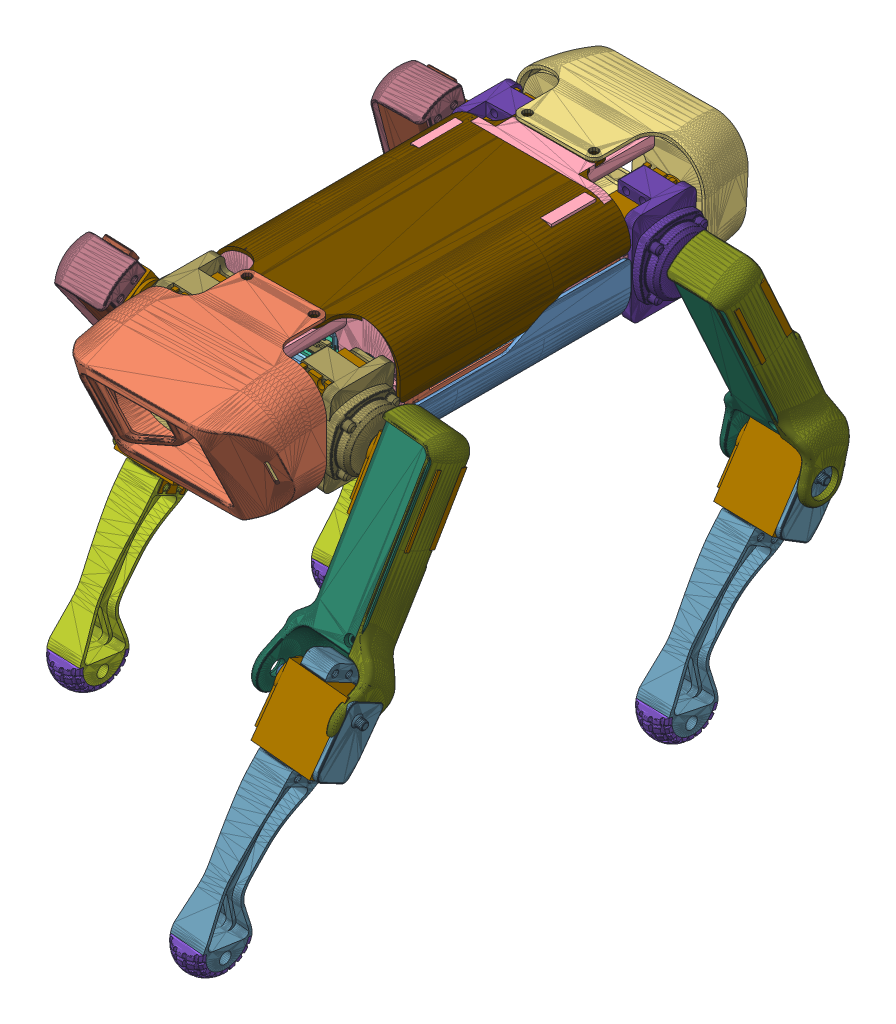
SolidWorks assembly robot_dog_jestson, configuration Default. Lengths in mm.
Overall size (261.86 298.31 449.5).
480 component instances, 93 part files, 20 mates.
Components (placement in the parent):
- torsol_with_jestson-1: torsol_with_jestson [Default] at (84.8958 -47.9637 220.9974) size (110.41 70.14 242.41)
  - R_side_plate-1: R_side_plate [Default] at (-145.3547 -0.5404 -42.0354) x (1 0 0) z (0 -1 0) size (6.5 130 29)
  - non-mega_L_side_plate_jetson-2: non-mega_L_side_plate_jetson [Default] at (-41.8547 39.5958 -42.0354) x (-1 0 0) z (0 1 0) size (6.5 130 29)
  - O_shoulder-1: O_shoulder [Default] at (-38.1905 81.6503 -93.0354) x (-1 0 0) z (0 -1 0) size (110 5.21 66)
  - I_shoulder_mg-1: I_shoulder_mg [Default] at (-38.6047 81.5958 -42.0354) x (-1 0 0) z (0 -1 0) size (110 51 70)
  - I_shoulder_mg-2: I_shoulder_mg [Default] at (-148.6047 81.4596 87.9646) x (1 0 0) z (0 -1 0) size (110 51 70)
  - O_shoulder-2: O_shoulder [Default] at (-148.6047 81.4596 138.9646) x (1 0 0) z (0 -1 0) size (110 5.21 66)
  - plate_with_jetson-1: plate_with_jetson [Default] at (-139.2728 38.0458 18.6623) x (-1 0 0) z (0 -1 0) size (107 130 44.9)
    - plate_jetson-1: plate_jetson [Default] at (-46.1681 -3.8023 -1.45) size (107 130 2.9)
    - Jetson nano_fixed.step-1: Jetson nano_fixed.step [Default] at (-69.1681 -65.6237 -1.45) x (0 1 0) z (0 0 -1) size (100 81.03 30.51)
      - 142-13449-1000-A02_ASM.step-1: 142-13449-1000-A02_ASM.step [Default] at origin size (100 81.03 23.19)
        - 142-13449-1000-A02.step-1: 142-13449-1000-A02.step [Default] at origin size (100 79 1.57)
        - 315-1109-000_1.step-1: 315-1109-000_1.step [Default] at (5.6 4.9 1.575) x (-1 0 0) z (0 0 1) size (4.5 3.5 0.8)
        - 0402_H040.step-1: 0402_H040.step [Default] at (8 -0.825 1.575) size (1 0.5 0.4)
        - 0402_H060.step-1: 0402_H060.step [Default] at (1 5 1.575) x (0 -1 0) z (0 0 1) size (1 0.5 0.6)
        - 0402_H040.step-2: 0402_H040.step [Default] at (9.9 -0.3 1.575) size (1 0.5 0.4)
        - 0402_H040.step-3: 0402_H040.step [Default] at (8.296 51.194 1.575) x (-1 0 0) z (0 0 1) size (1 0.5 0.4)
        - 0402_H040.step-4: 0402_H040.step [Default] at (76.2 36.9 1.575) x (-1 0 0) z (0 0 1) size (1 0.5 0.4)
        - 0402_H040.step-5: 0402_H040.step [Default] at (37.8 2.87 1.575) x (0 -1 0) z (0 0 1) size (1 0.5 0.4)
        - 0402_H040.step-6: 0402_H040.step [Default] at (38.6 2.87 1.575) x (0 -1 0) z (0 0 1) size (1 0.5 0.4)
        - 0402_H060.step-2: 0402_H060.step [Default] at (14.2 7.7 1.575) x (0 -1 0) z (0 0 1) size (1 0.5 0.6)
        - 0402_H040.step-7: 0402_H040.step [Default] at (64 27.5 1.575) x (-1 0 0) z (0 0 1) size (1 0.5 0.4)
        - 0402_H060.step-3: 0402_H060.step [Default] at (18.6 43.15 1.575) x (-1 0 0) z (0 0 1) size (1 0.5 0.6)
        - 0402_H060.step-4: 0402_H060.step [Default] at (65.5 52.8 1.575) x (0 1 0) z (0 0 1) size (1 0.5 0.6)
        - 0402_H060.step-5: 0402_H060.step [Default] at (64 28.4 1.575) x (-1 0 0) z (0 0 1) size (1 0.5 0.6)
        - 0402_H040.step-8: 0402_H040.step [Default] at (60.95 25.85 1.575) size (1 0.5 0.4)
        - 0402_H060.step-6: 0402_H060.step [Default] at (17.3 7.7 1.575) x (0 -1 0) z (0 0 1) size (1 0.5 0.6)
        - 0402_H060.step-7: 0402_H060.step [Default] at (18.6 7.7 1.575) x (0 -1 0) z (0 0 1) size (1 0.5 0.6)
        - 0402_H060.step-8: 0402_H060.step [Default] at (12.9 7.7 1.575) x (0 -1 0) z (0 0 1) size (1 0.5 0.6)
        - 0402_H060.step-9: 0402_H060.step [Default] at (80.9 37.7 1.575) x (-1 0 0) z (0 0 1) size (1 0.5 0.6)
        - 0402_H040.step-9: 0402_H040.step [Default] at (79.5 31.3 1.575) size (1 0.5 0.4)
        - 0402_H040.step-10: 0402_H040.step [Default] at (81 31.3 1.575) x (-1 0 0) z (0 0 1) size (1 0.5 0.4)
        - 0402_H060.step-10: 0402_H060.step [Default] at (79.3 37.7 1.575) size (1 0.5 0.6)
        - 0402_H060.step-11: 0402_H060.step [Default] at (74.8 4.05 1.575) x (-1 0 0) z (0 0 1) size (1 0.5 0.6)
        - 0402_H040.step-11: 0402_H040.step [Default] at (65.675 6.15 1.575) x (0 -1 0) z (0 0 1) size (1 0.5 0.4)
        - 0402_H060.step-12: 0402_H060.step [Default] at (67.7 6.85 1.575) x (0 1 0) z (0 0 1) size (1 0.5 0.6)
        - 0402_H040.step-12: 0402_H040.step [Default] at (64.475 5.8 1.575) x (-1 0 0) z (0 0 1) size (1 0.5 0.4)
        - 0402_H040.step-13: 0402_H040.step [Default] at (67.725 5.325 1.575) x (0 1 0) z (0 0 1) size (1 0.5 0.4)
        - 0402_H060.step-13: 0402_H060.step [Default] at (46.1 59.45 1.575) size (1 0.5 0.6)
        - 0402_H040.step-14: 0402_H040.step [Default] at (44.65 59.45 1.575) size (1 0.5 0.4)
        - 0402_H040.step-15: 0402_H040.step [Default] at (46.1 60.25 1.575) size (1 0.5 0.4)
        - 0402_H060.step-14: 0402_H060.step [Default] at (53.35 57.7 1.575) x (0 -1 0) z (0 0 1) size (1 0.5 0.6)
        - 0402_H040.step-16: 0402_H040.step [Default] at (47.6 59.45 1.575) size (1 0.5 0.4)
        - 0402_H040.step-17: 0402_H040.step [Default] at (48.4 60.25 1.575) size (1 0.5 0.4)
        - 0402_H040.step-18: 0402_H040.step [Default] at (47.7 58.325 1.575) x (0 1 0) z (0 0 1) size (1 0.5 0.4)
        - 0402_H060.step-15: 0402_H060.step [Default] at (46.5 58.65 1.575) x (-1 0 0) z (0 0 1) size (1 0.5 0.6)
        - 0402_H060.step-16: 0402_H060.step [Default] at (51.8 60.25 1.575) size (1 0.5 0.6)
        - 0402_H040.step-19: 0402_H040.step [Default] at (53.35 59.4 1.575) x (0 -1 0) z (0 0 1) size (1 0.5 0.4)
        - 0402_H040.step-20: 0402_H040.step [Default] at (50.2 60.25 1.575) x (-1 0 0) z (0 0 1) size (1 0.5 0.4)
        - 0402_H060.step-17: 0402_H060.step [Default] at (18.6 43.95 1.575) x (-1 0 0) z (0 0 1) size (1 0.5 0.6)
        - 0402_H060.step-18: 0402_H060.step [Default] at (52.75 2.9 1.575) x (0 -1 0) z (0 0 1) size (1 0.5 0.6)
        - 0402_H060.step-19: 0402_H060.step [Default] at (22.35 47.4 1.575) x (-1 0 0) z (0 0 1) size (1 0.5 0.6)
        - 0402_H060.step-20: 0402_H060.step [Default] at (20.55 47.4 1.575) x (-1 0 0) z (0 0 1) size (1 0.5 0.6)
        - 0402_H060.step-21: 0402_H060.step [Default] at (21.95 34.55 1.575) x (0 -1 0) z (0 0 1) size (1 0.5 0.6)
        - 0402_H060.step-22: 0402_H060.step [Default] at (21.05 34.55 1.575) x (0 -1 0) z (0 0 1) size (1 0.5 0.6)
        - 0402_H060.step-23: 0402_H060.step [Default] at (53.55 2.9 1.575) x (0 -1 0) z (0 0 1) size (1 0.5 0.6)
        - 0402_H060.step-24: 0402_H060.step [Default] at (25.4 54 1.575) x (-1 0 0) z (0 0 1) size (1 0.5 0.6)
        - 0402_H060.step-25: 0402_H060.step [Default] at (24 34.58 1.575) x (0 -1 0) z (0 0 1) size (1 0.5 0.6)
        - 0402_H040.step-21: 0402_H040.step [Default] at (55.6 2.95 1.575) x (0 -1 0) z (0 0 1) size (1 0.5 0.4)
        - 0402_H040.step-22: 0402_H040.step [Default] at (20.13 34.53 1.575) x (0 1 0) z (0 0 1) size (1 0.5 0.4)
        - 0402_H060.step-26: 0402_H060.step [Default] at (18.4 35.15 1.575) x (0 1 0) z (0 0 1) size (1 0.5 0.6)
        - 0402_H060.step-27: 0402_H060.step [Default] at (18.4 36.75 1.575) x (0 1 0) z (0 0 1) size (1 0.5 0.6)
        - 0402_H040.step-23: 0402_H040.step [Default] at (39.6 2.87 1.575) x (0 -1 0) z (0 0 1) size (1 0.5 0.4)
        - 0402_H040.step-24: 0402_H040.step [Default] at (40.4 2.87 1.575) x (0 -1 0) z (0 0 1) size (1 0.5 0.4)
        - 0402_H040.step-25: 0402_H040.step [Default] at (60.95 2.95 1.575) x (0 -1 0) z (0 0 1) size (1 0.5 0.4)
        - 0402_H040.step-26: 0402_H040.step [Default] at (60.15 2.95 1.575) x (0 -1 0) z (0 0 1) size (1 0.5 0.4)
        - 0402_H040.step-27: 0402_H040.step [Default] at (54.8 2.95 1.575) x (0 -1 0) z (0 0 1) size (1 0.5 0.4)
        - 0402_H040.step-28: 0402_H040.step [Default] at (31.6 54 1.575) size (1 0.5 0.4)
        - 0402_H040.step-29: 0402_H040.step [Default] at (27.4 54 1.575) size (1 0.5 0.4)
        - 0402_H040.step-30: 0402_H040.step [Default] at (29.6 54 1.575) x (-1 0 0) z (0 0 1) size (1 0.5 0.4)
        - 0402_H040.step-31: 0402_H040.step [Default] at (63.775 -14.475 1.575) size (1 0.5 0.4)
        - 0402_H040.step-32: 0402_H040.step [Default] at (63.775 -15.275 1.575) size (1 0.5 0.4)
        - 0402_H040.step-33: 0402_H040.step [Default] at (8.025 41.475 1.575) x (-1 0 0) z (0 0 1) size (1 0.5 0.4)
        - 0402_H060.step-28: 0402_H060.step [Default] at (63.95 1.25 1.575) x (0 1 0) z (0 0 1) size (1 0.5 0.6)
        - 0402_H060.step-29: 0402_H060.step [Default] at (2.95 54.05 1.575) x (0 1 0) z (0 0 1) size (1 0.5 0.6)
        - 0402_H040.step-34: 0402_H040.step [Default] at (92.2 -3.45 1.575) x (-1 0 0) z (0 0 1) size (1 0.5 0.4)
        - 0402_H060.step-30: 0402_H060.step [Default] at (32.85 7.7 1.575) x (0 -1 0) z (0 0 1) size (1 0.5 0.6)
        - 0402_H060.step-31: 0402_H060.step [Default] at (27.25 7.7 1.575) x (0 -1 0) z (0 0 1) size (1 0.5 0.6)
        - 0402_H060.step-32: 0402_H060.step [Default] at (31.25 7.7 1.575) x (0 -1 0) z (0 0 1) size (1 0.5 0.6)
        - 0402_H060.step-33: 0402_H060.step [Default] at (28.85 7.7 1.575) x (0 -1 0) z (0 0 1) size (1 0.5 0.6)
        - 0402_H060.step-34: 0402_H060.step [Default] at (32.05 7.7 1.575) x (0 -1 0) z (0 0 1) size (1 0.5 0.6)
        - 0402_H060.step-35: 0402_H060.step [Default] at (28.05 7.7 1.575) x (0 -1 0) z (0 0 1) size (1 0.5 0.6)
        - 0402_H060.step-36: 0402_H060.step [Default] at (30.45 7.7 1.575) x (0 -1 0) z (0 0 1) size (1 0.5 0.6)
        - 0402_H060.step-37: 0402_H060.step [Default] at (29.65 7.7 1.575) x (0 -1 0) z (0 0 1) size (1 0.5 0.6)
        - 0402_H060.step-38: 0402_H060.step [Default] at (24.65 6.41 1.575) x (0 -1 0) z (0 0 1) size (1 0.5 0.6)
        - 0402_H060.step-39: 0402_H060.step [Default] at (25.85 6.41 1.575) x (0 -1 0) z (0 0 1) size (1 0.5 0.6)
        - 0402_H060.step-40: 0402_H060.step [Default] at (4.2 36.5 1.575) x (0 1 0) z (0 0 1) size (1 0.5 0.6)
        - 0402_H060.step-41: 0402_H060.step [Default] at (89.7 4.7 1.575) x (0 -1 0) z (0 0 1) size (1 0.5 0.6)
        - 0402_H060.step-42: 0402_H060.step [Default] at (82.5 3.8 1.575) x (0 -1 0) z (0 0 1) size (1 0.5 0.6)
        - 0402_H060.step-43: 0402_H060.step [Default] at (12.65 49.7 1.575) size (1 0.5 0.6)
        - 0402_H060.step-44: 0402_H060.step [Default] at (11.2 50.15 1.575) x (0 -1 0) z (0 0 1) size (1 0.5 0.6)
        - 0402_H060.step-45: 0402_H060.step [Default] at (26.5 34.55 1.575) x (0 -1 0) z (0 0 1) size (1 0.5 0.6)
        - 0402_H060.step-46: 0402_H060.step [Default] at (29.9 34.5 1.575) x (0 -1 0) z (0 0 1) size (1 0.5 0.6)
        - 0402_H060.step-47: 0402_H060.step [Default] at (31.7 40.15 1.575) x (0 1 0) z (0 0 1) size (1 0.5 0.6)
        - 0402_H060.step-48: 0402_H060.step [Default] at (31.15 42.5 1.575) x (0 1 0) z (0 0 1) size (1 0.5 0.6)
        - 0402_H060.step-49: 0402_H060.step [Default] at (19.2 47.05 1.575) x (0 1 0) z (0 0 1) size (1 0.5 0.6)
        - 0402_H060.step-50: 0402_H060.step [Default] at (17.95 42 1.575) x (0 -1 0) z (0 0 1) size (1 0.5 0.6)
        - 0402_H060.step-51: 0402_H060.step [Default] at (27.3 48.25 1.575) x (0 1 0) z (0 0 1) size (1 0.5 0.6)
        - 0402_H060.step-52: 0402_H060.step [Default] at (31.7 37.85 1.575) x (0 -1 0) z (0 0 1) size (1 0.5 0.6)
        - 0402_H060.step-53: 0402_H060.step [Default] at (29.6 48.35 1.575) x (0 1 0) z (0 0 1) size (1 0.5 0.6)
        - 0402_H060.step-54: 0402_H060.step [Default] at (18.8 38.75 1.575) x (-1 0 0) z (0 0 1) size (1 0.5 0.6)
        - 0402_H060.step-55: 0402_H060.step [Default] at (18.7 57.2 1.575) x (0 -1 0) z (0 0 1) size (1 0.5 0.6)
        - 0402_H060.step-56: 0402_H060.step [Default] at (34.1 2.9 1.575) x (0 -1 0) z (0 0 1) size (1 0.5 0.6)
        - 0402_H060.step-57: 0402_H060.step [Default] at (35.8 2.9 1.575) x (0 -1 0) z (0 0 1) size (1 0.5 0.6)
        - 0402_H060.step-58: 0402_H060.step [Default] at (34.9 2.9 1.575) x (0 -1 0) z (0 0 1) size (1 0.5 0.6)
        - 0402_H060.step-59: 0402_H060.step [Default] at (36.6 2.9 1.575) x (0 -1 0) z (0 0 1) size (1 0.5 0.6)
        - 0402_H060.step-60: 0402_H060.step [Default] at (11.325 44.725 1.575) size (1 0.5 0.6)
        - 0402_H060.step-61: 0402_H060.step [Default] at (50.95 2.9 1.575) x (0 -1 0) z (0 0 1) size (1 0.5 0.6)
        - 0402_H060.step-62: 0402_H060.step [Default] at (51.75 2.9 1.575) x (0 -1 0) z (0 0 1) size (1 0.5 0.6)
        - 0402_H060.step-63: 0402_H060.step [Default] at (11.55 39.7 1.575) size (1 0.5 0.6)
        - 0402_H060.step-64: 0402_H060.step [Default] at (9.5 -8.5 1.575) x (-1 0 0) z (0 0 1) size (1 0.5 0.6)
        - 0402_H060.step-65: 0402_H060.step [Default] at (61.35 38.05 1.575) x (0 -1 0) z (0 0 1) size (1 0.5 0.6)
        - 0402_H060.step-66: 0402_H060.step [Default] at (60.55 38.05 1.575) x (0 -1 0) z (0 0 1) size (1 0.5 0.6)
        - 0402_H060.step-67: 0402_H060.step [Default] at (29.3 25.65 1.575) x (0 -1 0) z (0 0 1) size (1 0.5 0.6)
        - 0402_H060.step-68: 0402_H060.step [Default] at (63.3 56.2 1.575) x (0 1 0) z (0 0 1) size (1 0.5 0.6)
        - 0402_H060.step-69: 0402_H060.step [Default] at (20.5 54.2 1.575) size (1 0.5 0.6)
        - 0402_H060.step-70: 0402_H060.step [Default] at (60.1 32.15 1.575) x (0 1 0) z (0 0 1) size (1 0.5 0.6)
        - 0402_H060.step-71: 0402_H060.step [Default] at (60.9 32.15 1.575) x (0 1 0) z (0 0 1) size (1 0.5 0.6)
        - 0402_H060.step-72: 0402_H060.step [Default] at (18.6 44.85 1.575) size (1 0.5 0.6)
        - 0402_H060.step-73: 0402_H060.step [Default] at (18.6 45.65 1.575) size (1 0.5 0.6)
        - 0402_H060.step-74: 0402_H060.step [Default] at (18.1 27.25 1.575) size (1 0.5 0.6)
        - 0402_H060.step-75: 0402_H060.step [Default] at (15.1 7.7 1.575) x (0 -1 0) z (0 0 1) size (1 0.5 0.6)
        - 0402_H060.step-76: 0402_H060.step [Default] at (16.4 7.7 1.575) x (0 -1 0) z (0 0 1) size (1 0.5 0.6)
        - 0402_H060.step-77: 0402_H060.step [Default] at (20.8 7.7 1.575) x (0 -1 0) z (0 0 1) size (1 0.5 0.6)
        - 0402_H060.step-78: 0402_H060.step [Default] at (19.5 7.7 1.575) x (0 -1 0) z (0 0 1) size (1 0.5 0.6)
        - 0402_H060.step-79: 0402_H060.step [Default] at (21.9 2.8 1.575) size (1 0.5 0.6)
        - 0402_H060.step-80: 0402_H060.step [Default] at (12.75 29 1.575) size (1 0.5 0.6)
        - 0402_H060.step-81: 0402_H060.step [Default] at (10.225 5.1 1.575) size (1 0.5 0.6)
        - 0402_H060.step-82: 0402_H060.step [Default] at (22.8 27.65 1.575) x (0 1 0) z (0 0 1) size (1 0.5 0.6)
        - 0402_H060.step-83: 0402_H060.step [Default] at (18.85 25.15 1.575) x (0 -1 0) z (0 0 1) size (1 0.5 0.6)
        - 0402_H060.step-84: 0402_H060.step [Default] at (17.95 40.1 1.575) x (0 1 0) z (0 0 1) size (1 0.5 0.6)
        - 0402_H040.step-35: 0402_H040.step [Default] at (20.8 6.2 1.575) x (0 1 0) z (0 0 1) size (1 0.5 0.4)
        - 0402_H040.step-36: 0402_H040.step [Default] at (76 22.7 1.575) size (1 0.5 0.4)
        - 0402_H040.step-37: 0402_H040.step [Default] at (23.7 26.85 1.575) x (0 1 0) z (0 0 1) size (1 0.5 0.4)
        - 0402_H040.step-38: 0402_H040.step [Default] at (18 25.15 1.575) x (0 1 0) z (0 0 1) size (1 0.5 0.4)
        - 0402_H040.step-39: 0402_H040.step [Default] at (17.3 28.25 1.575) x (-1 0 0) z (0 0 1) size (1 0.5 0.4)
        - 0402_H040.step-40: 0402_H040.step [Default] at (13.15 4.2 1.575) x (0 -1 0) z (0 0 1) size (1 0.5 0.4)
        - 0402_H040.step-41: 0402_H040.step [Default] at (17.2 30.15 1.575) x (0 -1 0) z (0 0 1) size (1 0.5 0.4)
        - 0402_H040.step-42: 0402_H040.step [Default] at (14.2 6.2 1.575) x (0 1 0) z (0 0 1) size (1 0.5 0.4)
        - 0402_H040.step-43: 0402_H040.step [Default] at (12.9 6.2 1.575) x (0 1 0) z (0 0 1) size (1 0.5 0.4)
        - 0402_H040.step-44: 0402_H040.step [Default] at (15.1 6.2 1.575) x (0 1 0) z (0 0 1) size (1 0.5 0.4)
        - 0402_H040.step-45: 0402_H040.step [Default] at (16.4 6.2 1.575) x (0 1 0) z (0 0 1) size (1 0.5 0.4)
        - 0402_H040.step-46: 0402_H040.step [Default] at (19.5 6.2 1.575) x (0 1 0) z (0 0 1) size (1 0.5 0.4)
        - 0402_H040.step-47: 0402_H040.step [Default] at (17.3 6.2 1.575) x (0 1 0) z (0 0 1) size (1 0.5 0.4)
        - 0402_H040.step-48: 0402_H040.step [Default] at (18.6 6.2 1.575) x (0 1 0) z (0 0 1) size (1 0.5 0.4)
        - 0402_H040.step-49: 0402_H040.step [Default] at (24.2 24.55 1.575) x (0 1 0) z (0 0 1) size (1 0.5 0.4)
        - 0402_H040.step-50: 0402_H040.step [Default] at (23.5 54.9 1.575) x (0 1 0) z (0 0 1) size (1 0.5 0.4)
        - 0402_H040.step-51: 0402_H040.step [Default] at (13.2 39.75 1.575) x (-1 0 0) z (0 0 1) size (1 0.5 0.4)
        - 0402_H040.step-52: 0402_H040.step [Default] at (80.7 47.4 1.575) x (-1 0 0) z (0 0 1) size (1 0.5 0.4)
        - 0402_H040.step-53: 0402_H040.step [Default] at (77.5 22.7 1.575) x (-1 0 0) z (0 0 1) size (1 0.5 0.4)
        - 0402_H040.step-54: 0402_H040.step [Default] at (9.25 -12.75 1.575) x (-1 0 0) z (0 0 1) size (1 0.5 0.4)
        - 0402_H040.step-55: 0402_H040.step [Default] at (9.25 -11.95 1.575) x (-1 0 0) z (0 0 1) size (1 0.5 0.4)
        - 0402_H040.step-56: 0402_H040.step [Default] at (64.475 6.7 1.575) size (1 0.5 0.4)
        - 0402_H040.step-57: 0402_H040.step [Default] at (29.3 24 1.575) x (0 1 0) z (0 0 1) size (1 0.5 0.4)
        - 0402_H040.step-58: 0402_H040.step [Default] at (64.2 32.5 1.575) x (0 1 0) z (0 0 1) size (1 0.5 0.4)
        - 0402_H040.step-59: 0402_H040.step [Default] at (64.15 47.45 1.575) x (0 -1 0) z (0 0 1) size (1 0.5 0.4)
        - 0402_H040.step-60: 0402_H040.step [Default] at (64.2 31 1.575) x (0 -1 0) z (0 0 1) size (1 0.5 0.4)
        - 0402_H040.step-61: 0402_H040.step [Default] at (76.2 36.1 1.575) x (-1 0 0) z (0 0 1) size (1 0.5 0.4)
        - 0402_H040.step-62: 0402_H040.step [Default] at (78.4 45.15 1.575) size (1 0.5 0.4)
        - 0402_H040.step-63: 0402_H040.step [Default] at (81.7 38.6 1.575) size (1 0.5 0.4)
        - 0402_H040.step-64: 0402_H040.step [Default] at (81.7 39.4 1.575) size (1 0.5 0.4)
        - 0402_H040.step-65: 0402_H040.step [Default] at (59.35 51.825 1.575) size (1 0.5 0.4)
        - 0402_H040.step-66: 0402_H040.step [Default] at (60.825 51.825 1.575) x (-1 0 0) z (0 0 1) size (1 0.5 0.4)
        - 0402_H040.step-67: 0402_H040.step [Default] at (89.7 9.5 1.575) x (0 1 0) z (0 0 1) size (1 0.5 0.4)
        - 0402_H040.step-68: 0402_H040.step [Default] at (89.7 6.7 1.575) x (0 1 0) z (0 0 1) size (1 0.5 0.4)
        - 0402_H040.step-69: 0402_H040.step [Default] at (3.9 34.2 1.575) x (0 -1 0) z (0 0 1) size (1 0.5 0.4)
        - 0402_H040.step-70: 0402_H040.step [Default] at (5.1 35 1.575) x (0 1 0) z (0 0 1) size (1 0.5 0.4)
        - 0402_H040.step-71: 0402_H040.step [Default] at (32.85 5.81 1.575) x (0 -1 0) z (0 0 1) size (1 0.5 0.4)
        - 0402_H040.step-72: 0402_H040.step [Default] at (32.05 5.81 1.575) x (0 -1 0) z (0 0 1) size (1 0.5 0.4)
        - 0402_H040.step-73: 0402_H040.step [Default] at (27.25 5.81 1.575) x (0 -1 0) z (0 0 1) size (1 0.5 0.4)
        - 0402_H040.step-74: 0402_H040.step [Default] at (28.05 5.81 1.575) x (0 -1 0) z (0 0 1) size (1 0.5 0.4)
        - 0402_H040.step-75: 0402_H040.step [Default] at (31.25 5.81 1.575) x (0 -1 0) z (0 0 1) size (1 0.5 0.4)
        - 0402_H040.step-76: 0402_H040.step [Default] at (30.45 5.81 1.575) x (0 -1 0) z (0 0 1) size (1 0.5 0.4)
        - 0402_H040.step-77: 0402_H040.step [Default] at (28.85 5.81 1.575) x (0 -1 0) z (0 0 1) size (1 0.5 0.4)
        - 0402_H040.step-78: 0402_H040.step [Default] at (29.65 5.81 1.575) x (0 -1 0) z (0 0 1) size (1 0.5 0.4)
        - 0402_H040.step-79: 0402_H040.step [Default] at (13.5 52.9 1.575) x (-1 0 0) z (0 0 1) size (1 0.5 0.4)
        - 0402_H040.step-80: 0402_H040.step [Default] at (22.35 4 1.575) x (0 -1 0) z (0 0 1) size (1 0.5 0.4)
        - 0402_H040.step-81: 0402_H040.step [Default] at (21.55 4 1.575) x (0 1 0) z (0 0 1) size (1 0.5 0.4)
        - 0402_H040.step-82: 0402_H040.step [Default] at (25.85 4.9 1.575) x (0 -1 0) z (0 0 1) size (1 0.5 0.4)
        - 0402_H040.step-83: 0402_H040.step [Default] at (11.8 52.9 1.575) size (1 0.5 0.4)
        - 0402_H040.step-84: 0402_H040.step [Default] at (9.432 51.594 1.575) x (0 -1 0) z (0 0 1) size (1 0.5 0.4)
        - 0402_H040.step-85: 0402_H040.step [Default] at (8.975 50.3 1.575) size (1 0.5 0.4)
        - 0402_H040.step-86: 0402_H040.step [Default] at (82.8 -5.3 1.575) x (-1 0 0) z (0 0 1) size (1 0.5 0.4)
        - 0402_H040.step-87: 0402_H040.step [Default] at (82.4 -11.6 1.575) x (-1 0 0) z (0 0 1) size (1 0.5 0.4)
        - 0402_H040.step-88: 0402_H040.step [Default] at (22.8 26.05 1.575) x (0 1 0) z (0 0 1) size (1 0.5 0.4)
        - 0402_H040.step-89: 0402_H040.step [Default] at (20.8 28.25 1.575) size (1 0.5 0.4)
        - 0402_H040.step-90: 0402_H040.step [Default] at (20.8 24.65 1.575) x (-1 0 0) z (0 0 1) size (1 0.5 0.4)
        - 0402_H040.step-91: 0402_H040.step [Default] at (18.1 26.45 1.575) size (1 0.5 0.4)
        - 0402_H040.step-92: 0402_H040.step [Default] at (24.65 8.41 1.575) x (0 1 0) z (0 0 1) size (1 0.5 0.4)
        - 0402_H040.step-93: 0402_H040.step [Default] at (25.85 8.41 1.575) x (0 1 0) z (0 0 1) size (1 0.5 0.4)
        - 0402_H040.step-94: 0402_H040.step [Default] at (3.8 54.4 1.575) x (0 -1 0) z (0 0 1) size (1 0.5 0.4)
        - 0402_H040.step-95: 0402_H040.step [Default] at (2.45 44.45 1.575) x (0 -1 0) z (0 0 1) size (1 0.5 0.4)
        - 0402_H040.step-96: 0402_H040.step [Default] at (24.65 4.9 1.575) x (0 1 0) z (0 0 1) size (1 0.5 0.4)
        - 0402_H040.step-97: 0402_H040.step [Default] at (22.15 7.6 1.575) x (-1 0 0) z (0 0 1) size (1 0.5 0.4)
        - 0402_H040.step-98: 0402_H040.step [Default] at (79.2 47.4 1.575) size (1 0.5 0.4)
        - 0402_H040.step-99: 0402_H040.step [Default] at (19 28.25 1.575) size (1 0.5 0.4)
        - 0402_H040.step-100: 0402_H040.step [Default] at (9.65 9.7 1.575) x (0 -1 0) z (0 0 1) size (1 0.5 0.4)
        - 0402_H040.step-101: 0402_H040.step [Default] at (28.35 34.45 1.575) x (0 1 0) z (0 0 1) size (1 0.5 0.4)
        - 0402_H040.step-102: 0402_H040.step [Default] at (25.2 34.55 1.575) x (0 1 0) z (0 0 1) size (1 0.5 0.4)
        - 0402_H040.step-103: 0402_H040.step [Default] at (10.625 6.35 1.575) x (0 -1 0) z (0 0 1) size (1 0.5 0.4)
        - 0402_H040.step-104: 0402_H040.step [Default] at (9.825 6.35 1.575) x (0 1 0) z (0 0 1) size (1 0.5 0.4)
        - 0402_H040.step-105: 0402_H040.step [Default] at (4.775 42.975 1.575) x (0 1 0) z (0 0 1) size (1 0.5 0.4)
        - 0402_H040.step-106: 0402_H040.step [Default] at (19.8 32.9 1.575) x (-1 0 0) z (0 0 1) size (1 0.5 0.4)
        - 0402_H040.step-107: 0402_H040.step [Default] at (22.35 24.65 1.575) x (-1 0 0) z (0 0 1) size (1 0.5 0.4)
        - 0402_H040.step-108: 0402_H040.step [Default] at (62.4 54.7 1.575) size (1 0.5 0.4)
        - 0402_H040.step-109: 0402_H040.step [Default] at (62.2 60.05 1.575) x (-1 0 0) z (0 0 1) size (1 0.5 0.4)
        - 0402_H040.step-110: 0402_H040.step [Default] at (23.5 57.5 1.575) x (0 1 0) z (0 0 1) size (1 0.5 0.4)
        - 0402_H040.step-111: 0402_H040.step [Default] at (12.8 44.725 1.575) size (1 0.5 0.4)
        - 0402_H040.step-112: 0402_H040.step [Default] at (21.8 31.45 1.575) x (0 1 0) z (0 0 1) size (1 0.5 0.4)
        - 0402_H040.step-113: 0402_H040.step [Default] at (19.25 34.55 1.575) x (0 1 0) z (0 0 1) size (1 0.5 0.4)
        - 0402_H040.step-114: 0402_H040.step [Default] at (0.95 41.55 1.575) size (1 0.5 0.4)
        - 0402_H040.step-115: 0402_H040.step [Default] at (64.1 58 1.575) x (0 1 0) z (0 0 1) size (1 0.5 0.4)
        - 0402_H040.step-116: 0402_H040.step [Default] at (63.3 58 1.575) x (0 -1 0) z (0 0 1) size (1 0.5 0.4)
        - 0402_H040.step-117: 0402_H040.step [Default] at (63.55 59.7 1.575) x (0 -1 0) z (0 0 1) size (1 0.5 0.4)
        - 0402_H060.step-85: 0402_H060.step [Default] at (71.175 4 1.575) x (-1 0 0) z (0 0 1) size (1 0.5 0.6)
        - 0402_H040.step-118: 0402_H040.step [Default] at (86.6 -5.6 1.575) x (0 1 0) z (0 0 1) size (1 0.5 0.4)
        - 0402_H040.step-119: 0402_H040.step [Default] at (85.8 -5.3 1.575) x (0 1 0) z (0 0 1) size (1 0.5 0.4)
        - 0402_H040.step-120: 0402_H040.step [Default] at (10.25 51.6 1.575) x (0 1 0) z (0 0 1) size (1 0.5 0.4)
        - 0402_H040.step-121: 0402_H040.step [Default] at (80.5 28.55 1.575) size (1 0.5 0.4)
        - 0402_H040.step-122: 0402_H040.step [Default] at (13.95 4.2 1.575) x (0 -1 0) z (0 0 1) size (1 0.5 0.4)
        - 0402_H040.step-123: 0402_H040.step [Default] at (15.35 4.2 1.575) x (0 -1 0) z (0 0 1) size (1 0.5 0.4)
        - 0402_H040.step-124: 0402_H040.step [Default] at (16.15 4.2 1.575) x (0 -1 0) z (0 0 1) size (1 0.5 0.4)
        - 0402_H040.step-125: 0402_H040.step [Default] at (20.55 4.2 1.575) x (0 -1 0) z (0 0 1) size (1 0.5 0.4)
        - 0402_H040.step-126: 0402_H040.step [Default] at (19.75 4.2 1.575) x (0 -1 0) z (0 0 1) size (1 0.5 0.4)
        - 0402_H040.step-127: 0402_H040.step [Default] at (17.6 4.2 1.575) x (0 -1 0) z (0 0 1) size (1 0.5 0.4)
        - 0402_H040.step-128: 0402_H040.step [Default] at (18.4 4.2 1.575) x (0 -1 0) z (0 0 1) size (1 0.5 0.4)
        - 0402_H060.step-86: 0402_H060.step [Default] at (64.25 -13.325 1.575) x (0 -1 0) z (0 0 1) size (1 0.5 0.6)
        - 0402_H060.step-87: 0402_H060.step [Default] at (64.225 -11.825 1.575) x (0 1 0) z (0 0 1) size (1 0.5 0.6)
        - 0402_H040.step-129: 0402_H040.step [Default] at (63.8 -6.85 1.575) x (0 1 0) z (0 0 1) size (1 0.5 0.4)
        - 0402_H040.step-130: 0402_H040.step [Default] at (81.7 41.95 1.575) size (1 0.5 0.4)
        - 0402_H040.step-131: 0402_H040.step [Default] at (87.75 -6 1.575) x (-1 0 0) z (0 0 1) size (1 0.5 0.4)
        - 0402_H040.step-132: 0402_H040.step [Default] at (82.4 -13.6 1.575) x (-1 0 0) z (0 0 1) size (1 0.5 0.4)
        - 0402_H060.step-88: 0402_H060.step [Default] at (91.75 -5.95 1.575) size (1 0.5 0.6)
        - 0402_H040.step-133: 0402_H040.step [Default] at (3.65 49.25 1.575) x (0 -1 0) z (0 0 1) size (1 0.5 0.4)
        - 0402_H040.step-134: 0402_H040.step [Default] at (2.45 49.25 1.575) x (0 1 0) z (0 0 1) size (1 0.5 0.4)
        - 0402_H040.step-135: 0402_H040.step [Default] at (90.75 -1.45 1.575) x (-1 0 0) z (0 0 1) size (1 0.5 0.4)
        - 0402_H040.step-136: 0402_H040.step [Default] at (8.45 39.55 1.575) x (0 -1 0) z (0 0 1) size (1 0.5 0.4)
        - 0402_H060.step-89: 0402_H060.step [Default] at (8.85 -5.25 1.575) x (-1 0 0) z (0 0 1) size (1 0.5 0.6)
        - 0402_H040.step-137: 0402_H040.step [Default] at (18.6 32.55 1.575) x (0 1 0) z (0 0 1) size (1 0.5 0.4)
        - 0402_H060.step-90: 0402_H060.step [Default] at (4.5 44.45 1.575) x (0 1 0) z (0 0 1) size (1 0.5 0.6)
        - 0402_H040.step-138: 0402_H040.step [Default] at (8.35 2.75 1.575) size (1 0.5 0.4)
        - 0402_H040.step-139: 0402_H040.step [Default] at (9.4 1.95 1.575) size (1 0.5 0.4)
        - 0402_H040.step-140: 0402_H040.step [Default] at (8.2 1.55 1.575) x (0 1 0) z (0 0 1) size (1 0.5 0.4)
        - 0402_H060.step-91: 0402_H060.step [Default] at (8.5 3.875 1.575) x (0 -1 0) z (0 0 1) size (1 0.5 0.6)
        - 0402_H060.step-92: 0402_H060.step [Default] at (-0.8 41.5 1.575) x (-1 0 0) z (0 0 1) size (1 0.5 0.6)
        - 0402_H040.step-141: 0402_H040.step [Default] at (-1.35 7.75 1.575) size (1 0.5 0.4)
        - 0402_H040.step-142: 0402_H040.step [Default] at (8 0.425 1.575) size (1 0.5 0.4)
        - 0402_H040.step-143: 0402_H040.step [Default] at (67.9 4.025 1.575) x (-1 0 0) z (0 0 1) size (1 0.5 0.4)
        - 0402_H040.step-144: 0402_H040.step [Default] at (60.6 60.05 1.575) x (-1 0 0) z (0 0 1) size (1 0.5 0.4)
        - 0402_H040.step-145: 0402_H040.step [Default] at (72.85 4 1.575) x (-1 0 0) z (0 0 1) size (1 0.5 0.4)
        - 0402_H040.step-146: 0402_H040.step [Default] at (64.8 59.35 1.575) size (1 0.5 0.4)
        - 0402_H040.step-147: 0402_H040.step [Default] at (7.2 7.3 1.575) size (1 0.5 0.4)
        - 0402_H040.step-148: 0402_H040.step [Default] at (8.5 5.35 1.575) x (0 1 0) z (0 0 1) size (1 0.5 0.4)
        - 0402_H040.step-149: 0402_H040.step [Default] at (8.475 7.075 1.575) x (0 1 0) z (0 0 1) size (1 0.5 0.4)
        - VIRTUAL_SHORT.step-1: VIRTUAL_SHORT.step [Default] at (23.5 32.9 1.575) x (0 1 0) z (0 0 1) size (0.25 0.25 1)
        - VIRTUAL_SHORT.step-2: VIRTUAL_SHORT.step [Default] at (26.85 32.85 1.575) x (0 1 0) z (0 0 1) size (0.25 0.25 1)
        - VIRTUAL_SHORT.step-3: VIRTUAL_SHORT.step [Default] at (30.6 33.8 1.575) x (0 1 0) z (0 0 1) size (0.25 0.25 1)
        - VIRTUAL_SHORT.step-4: VIRTUAL_SHORT.step [Default] at (32.65 39.75 1.575) x (-1 0 0) z (0 0 1) size (0.25 0.25 1)
        - VIRTUAL_SHORT.step-5: VIRTUAL_SHORT.step [Default] at (31.85 42.1 1.575) x (-1 0 0) z (0 0 1) size (0.25 0.25 1)
        - VIRTUAL_SHORT.step-6: VIRTUAL_SHORT.step [Default] at (17.35 42.4 1.575) size (0.25 0.25 1)
        - VIRTUAL_SHORT.step-7: VIRTUAL_SHORT.step [Default] at (18.6 46.6 1.575) size (0.25 0.25 1)
        - VIRTUAL_SHORT.step-8: VIRTUAL_SHORT.step [Default] at (20.9 32.9 1.575) x (0 1 0) z (0 0 1) size (0.25 0.25 1)
        - VIRTUAL_SHORT.step-9: VIRTUAL_SHORT.step [Default] at (28.6 48.25 1.575) x (0 -1 0) z (0 0 1) size (0.25 0.25 1)
        - VIRTUAL_SHORT.step-10: VIRTUAL_SHORT.step [Default] at (27.1 49.35 1.575) x (0 -1 0) z (0 0 1) size (0.25 0.25 1)
        - VIRTUAL_SHORT.step-11: VIRTUAL_SHORT.step [Default] at (22.1 32.95 1.575) x (-1 0 0) z (0 0 1) size (0.25 0.25 1)
        - VIRTUAL_SHORT.step-12: VIRTUAL_SHORT.step [Default] at (32.65 38.25 1.575) x (-1 0 0) z (0 0 1) size (0.25 0.25 1)
        - VIRTUAL_SHORT.step-13: VIRTUAL_SHORT.step [Default] at (30.3 48 1.575) x (-1 0 0) z (0 0 1) size (0.25 0.25 1)
        - VIRTUAL_SHORT.step-14: VIRTUAL_SHORT.step [Default] at (17.15 38.95 1.575) size (0.25 0.25 1)
        - VIRTUAL_SHORT.step-15: VIRTUAL_SHORT.step [Default] at (17.15 39.7 1.575) size (0.25 0.25 1)
        - VIRTUAL_SHORT.step-16: VIRTUAL_SHORT.step [Default] at (76.175 4.1 1.575) x (-1 0 0) z (0 0 1) size (0.25 0.25 1)
        - 064-0377-000_2.step-1: 064-0377-000_2.step [Default] at (2 -4.75 1.575) x (0 -1 0) z (0 0 1) size (14.63 10.08 14.5)
        - 074-0117-000_2.step-1: 074-0117-000_2.step [Default] at (0.254 14.3 1.575) size (5.08 2.54 11.66)
        - 090-0096-000_1.step-1: 090-0096-000_1.step [Default] at (3.45 44.4 1.575) x (0 -1 0) z (0 0 1) size (1.2 0.6 0.4)
        - 090-0309-000_1.step-1: 090-0309-000_1.step [Default] at (-1.65 8.7 1.575) x (-1 0 0) z (0 0 1) size (1.2 0.6 0.4)
        - 115-1232-000_2.step-1: 115-1232-000_2.step [Default] at (1.25 6.5 1.575) x (-1 0 0) z (0 0 1) size (0.9 0.9 0.33)
        - 074-0102-000_4.step-1: 074-0102-000_4.step [Default] at (0.254 44.36 1.575) x (0 1 0) z (0 0 1) size (10.16 5.08 11.6)
        - 064-0400-000_1.step-1: 064-0400-000_1.step [Default] at (73.75 7.77 1.575) size (10.16 5.8 13.5)
        - MEC_STANDOFF_PTH_620C380P.step-1: MEC_STANDOFF_PTH_620C380P.step [Default] at (40.276 40.3 1.575) x (0 1 0) z (0 0 1) size (6.2 6.2 0.73)
        - 090-0231-000_1.step-1: 090-0231-000_1.step [Default] at (35.3 0.7 1.575) x (-1 0 0) z (0 0 1) size (2.5 1.55 0.55)
        - 090-0231-000_1.step-2: 090-0231-000_1.step [Default] at (52.25 0.7 1.575) x (-1 0 0) z (0 0 1) size (2.5 1.55 0.55)
        - 090-0231-000_1.step-3: 090-0231-000_1.step [Default] at (56.05 0.7 1.575) size (2.5 1.55 0.55)
        - 090-0231-000_1.step-4: 090-0231-000_1.step [Default] at (59.65 0.7 1.575) size (2.5 1.55 0.55)
        - 090-0231-000_1.step-5: 090-0231-000_1.step [Default] at (39.1 0.7 1.575) size (2.5 1.55 0.55)
        - 090-0231-000_1.step-6: 090-0231-000_1.step [Default] at (43.1 0.7 1.575) size (2.5 1.55 0.55)
        - 090-0231-000_1.step-7: 090-0231-000_1.step [Default] at (14.6 1.8 1.575) size (2.5 1.55 0.55)
        - 090-0231-000_1.step-8: 090-0231-000_1.step [Default] at (19.1 1.8 1.575) size (2.5 1.55 0.55)
        - 090-0231-000_1.step-9: 090-0231-000_1.step [Default] at (22.5 1.4 1.575) size (2.5 1.55 0.55)
        - 090-0231-000_1.step-10: 090-0231-000_1.step [Default] at (28.45 3.35 1.575) size (2.5 1.55 0.55)
        - 090-0231-000_1.step-11: 090-0231-000_1.step [Default] at (31.65 3.35 1.575) size (2.5 1.55 0.55)
        - 074-0223-000_2.step-1: 074-0223-000_2.step [Default] at (5.85 53.25 1.575) x (0 1 0) z (0 0 1) size (15.24 2.54 11.6)
        - 131-0832-000_2.step-1: 131-0832-000_2.step [Default] at (56.3 54.7 1.575) x (0 -1 0) z (0 0 1) size (4.96 4.06 1.8)
        - 115-0836-000_1.step-1: 115-0836-000_1.step [Default] at (21.1 56.6 1.575) size (2.9 3.58 1.45)
        - 115-0836-000_1.step-2: 115-0836-000_1.step [Default] at (11.8 42.3 1.575) size (2.9 3.58 1.45)
        - 315-0620-000_1.step-1: 315-0620-000_1.step [Default] at (72.1 53.4 1.575) x (0 -1 0) z (0 0 1) size (2.9 3.58 1.1)
        - 315-1062-000_1.step-1: 315-1062-000_1.step [Default] at (26.8 25.15 1.575) x (0 -1 0) z (0 0 1) size (2.9 3.58 1.45)
        - 170-0285-000_1.step-1: 170-0285-000_1.step [Default] at (28.72 57.28 1.575) x (0 1 0) z (0 0 1) size (4.9 7.21 1.75)
        - 115-0138-000_1.step-1: 115-0138-000_1.step [Default] at (9.15 48.55 1.575) x (0 1 0) z (0 0 1) size (2 2.88 1.1)
        - 115-1821-000_1.step-1: 115-1821-000_1.step [Default] at (3.3 40.8 1.575) x (-1 0 0) z (0 0 1) size (2 2.88 1.1)
